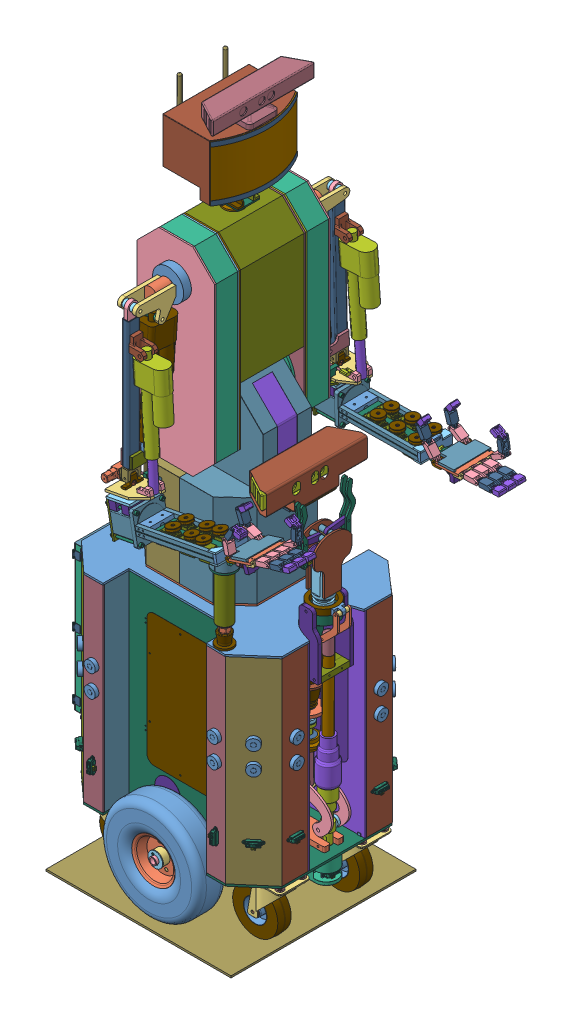
SolidWorks assembly sorbot, configuration По умолчанию. Lengths in mm.
Overall size (793.33 1880.98 665.85).
1182 component instances, 374 part files, 1522 mates.
Components (placement in the parent):
- wheel-1: wheel [По умолчанию] at (-13.022 1.4469 17.7637) size (270 270 80)
  - wheel.chamber-1: wheel.chamber [По умолчанию] at (6.3301 10.4899 0) size (270 270 80)
  - wheel.metal.front-1: wheel.metal.front [По умолчанию] at (6.3301 10.4899 42.7077) x (-0.311346 0.950297 0) z (0.950297 0.311346 0) size (117.48 26.95 117.48)
  - wheel.metal.internal-1: wheel.metal.internal [По умолчанию] at (6.3301 10.4899 36.3681) x (0.950297 0.311346 0) z (-0.311346 0.950297 0) size (117.48 60 117.48)
- wheel-2: wheel [По умолчанию] at (1.0599 2.4489 -290) x (-0.989924 -0.141601 0) z (0 0 -1) size (270 270 80)
  - wheel.chamber-1: wheel.chamber [По умолчанию] at (6.3301 10.4899 0) size (270 270 80)
  - wheel.metal.front-1: wheel.metal.front [По умолчанию] at (6.3301 10.4899 42.7077) x (-0.311346 0.950297 0) z (0.950297 0.311346 0) size (117.48 26.95 117.48)
  - wheel.metal.internal-1: wheel.metal.internal [По умолчанию] at (6.3301 10.4899 36.3681) x (0.950297 0.311346 0) z (-0.311346 0.950297 0) size (117.48 60 117.48)
- wheel.axis-1: wheel.axis [По умолчанию] at (-6.6918 11.9368 88.1319) x (-0.923728 -0.383049 0) z (0 0 -1) size (20 20 450)
- wheel.washer-1: wheel.washer [По умолчанию] at (-6.6918 11.9368 79.1319) size (40 40 2)
- wheel.washer-2: wheel.washer [По умолчанию] at (-6.6918 11.9368 -353.3681) size (40 40 2)
- wheel.axis.splint-1: wheel.axis.splint [По умолчанию] at (-51.8409 -4.2239 -121.73) x (0.909121 0.380793 -0.168805) z (0.181229 0.003281 0.983435) size (4.99 27.52 1.94)
- wheel.axis.splint-2: wheel.axis.splint [По умолчанию] at (-119.6931 -47.4576 -189.7376) x (-0.699932 -0.282835 -0.65582) z (0.605814 0.251217 -0.754904) size (4.99 27.52 1.94)
- wheel.disk-1: wheel.disk [По умолчанию] at (-6.6918 11.9368 -326.3681) size (86 86 70)
- gearmotor-1: gearmotor [По умолчанию] at (53.2168 119.2767 -131.0001) x (0.993251 -0.115983 0) z (0 0 1) size (79 79 282)
- wheel.bearing-1: wheel.bearing [По умолчанию] at (-6.6918 11.9368 -263.3681) x (0.993854 -0.110698 0) z (0 0 1) size (32 32 7)
- wheel.stop.bearing-2: wheel.stop.bearing [По умолчанию] at (-3.289 9.2452 -250.3457) size (52.27 52.27 14.02)
  - wheel.stop.bearing.p1-1: wheel.stop.bearing.p1 [По умолчанию] at (-3.4029 2.6916 -6.0224) size (40 40 4)
  - wheel.stop.bearing.p2-1: wheel.stop.bearing.p2 [По умолчанию] at (-3.421 17.5634 1.5621) size (7 7 7)
  - wheel.stop.bearing.p1-2: wheel.stop.bearing.p1 [По умолчанию] at (-3.4029 2.6916 8) x (-0.923728 -0.383049 0) z (0 0 -1) size (40 40 4)
  - wheel.stop.bearing.p2-3: wheel.stop.bearing.p2 [По умолчанию] at (4.0173 15.58 1.5621) x (0.866025 -0.5 0) z (0 0 1) size (7 7 7)
  - wheel.stop.bearing.p2-4: wheel.stop.bearing.p2 [По умолчанию] at (9.4674 10.1432 1.5621) x (0.5 -0.866025 0) z (0 0 1) size (7 7 7)
  - wheel.stop.bearing.p2-5: wheel.stop.bearing.p2 [По умолчанию] at (11.469 2.7097 1.5621) x (0 -1 0) z (0 0 1) size (7 7 7)
  - wheel.stop.bearing.p2-6: wheel.stop.bearing.p2 [По умолчанию] at (9.4856 -4.7286 1.5621) x (-0.5 -0.866025 0) z (0 0 1) size (7 7 7)
  - wheel.stop.bearing.p2-7: wheel.stop.bearing.p2 [По умолчанию] at (4.0488 -10.1787 1.5621) x (-0.866025 -0.5 0) z (0 0 1) size (7 7 7)
  - wheel.stop.bearing.p2-8: wheel.stop.bearing.p2 [По умолчанию] at (-3.3847 -12.1802 1.5621) x (-1 0 0) z (0 0 1) size (7 7 7)
  - wheel.stop.bearing.p2-9: wheel.stop.bearing.p2 [По умолчанию] at (-10.8231 -10.1969 1.5621) x (-0.866025 0.5 0) z (0 0 1) size (7 7 7)
  - wheel.stop.bearing.p2-10: wheel.stop.bearing.p2 [По умолчанию] at (-16.2732 -4.76 1.5621) x (-0.5 0.866025 0) z (0 0 1) size (7 7 7)
  - wheel.stop.bearing.p2-11: wheel.stop.bearing.p2 [По умолчанию] at (-18.2747 2.6734 1.5621) x (0 1 0) z (0 0 1) size (7 7 7)
  - wheel.stop.bearing.p2-12: wheel.stop.bearing.p2 [По умолчанию] at (-16.2913 10.1118 1.5621) x (0.5 0.866025 0) z (0 0 1) size (7 7 7)
  - wheel.stop.bearing.p2-13: wheel.stop.bearing.p2 [По умолчанию] at (-10.8545 15.5619 1.5621) x (0.866025 0.5 0) z (0 0 1) size (7 7 7)
- sproket.initial-1: sproket.initial [По умолчанию] at (53.2168 119.2767 -271.5001) x (0.999977 0.00678 0) z (0 0 1) size (82.09 81.83 4.4)
- gearmotor.sprocket.wheel.disk-1: gearmotor.sprocket.wheel.disk [По умолчанию] at (53.2168 119.2767 -276.8747) x (0.999997 -0.002459 0) z (0 0 1) size (68 68 28.87)
- sprocket-1: sprocket [По умолчанию] at (-6.6918 11.9368 -271.3681) size (82.09 81.83 3)
- bottom-2: bottom [По умолчанию] at (-6.1674 46.4368 -211.0406) size (543.13 5.5 438.63)
- wheel.axis.frame-3: wheel.axis.frame [По умолчанию] at (43.3082 10.4368 -242.3457) x (-1 0 0) z (0 0 1) size (126 65.5 38)
- accumulator1-1: accumulator1 [По умолчанию] at (-188.4596 154.9368 -137.8821) x (0 0 1) z (-1 0 0) size (232 218.1 175)
- wheel.disk-2: wheel.disk [По умолчанию] at (-6.6918 11.9368 54.1319) x (-0.923728 -0.383049 0) z (0 0 -1) size (86 86 70)
- wheel.bearing-2: wheel.bearing [По умолчанию] at (-6.6918 11.9368 -15.8681) size (32 32 7)
- wheel.stop.bearing-3: wheel.stop.bearing [По умолчанию] at (-3.289 9.2452 -23.8681) size (52.27 52.27 14.02)
  - wheel.stop.bearing.p1-1: wheel.stop.bearing.p1 [По умолчанию] at (-3.4029 2.6916 -6.0224) size (40 40 4)
  - wheel.stop.bearing.p2-1: wheel.stop.bearing.p2 [По умолчанию] at (-3.421 17.5634 1.5621) size (7 7 7)
  - wheel.stop.bearing.p1-2: wheel.stop.bearing.p1 [По умолчанию] at (-3.4029 2.6916 8) x (-0.923728 -0.383049 0) z (0 0 -1) size (40 40 4)
  - wheel.stop.bearing.p2-3: wheel.stop.bearing.p2 [По умолчанию] at (4.0173 15.58 1.5621) x (0.866025 -0.5 0) z (0 0 1) size (7 7 7)
  - wheel.stop.bearing.p2-4: wheel.stop.bearing.p2 [По умолчанию] at (9.4674 10.1432 1.5621) x (0.5 -0.866025 0) z (0 0 1) size (7 7 7)
  - wheel.stop.bearing.p2-5: wheel.stop.bearing.p2 [По умолчанию] at (11.469 2.7097 1.5621) x (0 -1 0) z (0 0 1) size (7 7 7)
  - wheel.stop.bearing.p2-6: wheel.stop.bearing.p2 [По умолчанию] at (9.4856 -4.7286 1.5621) x (-0.5 -0.866025 0) z (0 0 1) size (7 7 7)
  - wheel.stop.bearing.p2-7: wheel.stop.bearing.p2 [По умолчанию] at (4.0488 -10.1787 1.5621) x (-0.866025 -0.5 0) z (0 0 1) size (7 7 7)
  - wheel.stop.bearing.p2-8: wheel.stop.bearing.p2 [По умолчанию] at (-3.3847 -12.1802 1.5621) x (-1 0 0) z (0 0 1) size (7 7 7)
  - wheel.stop.bearing.p2-9: wheel.stop.bearing.p2 [По умолчанию] at (-10.8231 -10.1969 1.5621) x (-0.866025 0.5 0) z (0 0 1) size (7 7 7)
  - wheel.stop.bearing.p2-10: wheel.stop.bearing.p2 [По умолчанию] at (-16.2732 -4.76 1.5621) x (-0.5 0.866025 0) z (0 0 1) size (7 7 7)
  - wheel.stop.bearing.p2-11: wheel.stop.bearing.p2 [По умолчанию] at (-18.2747 2.6734 1.5621) x (0 1 0) z (0 0 1) size (7 7 7)
  - wheel.stop.bearing.p2-12: wheel.stop.bearing.p2 [По умолчанию] at (-16.2913 10.1118 1.5621) x (0.5 0.866025 0) z (0 0 1) size (7 7 7)
  - wheel.stop.bearing.p2-13: wheel.stop.bearing.p2 [По умолчанию] at (-10.8545 15.5619 1.5621) x (0.866025 0.5 0) z (0 0 1) size (7 7 7)
- wheel.axis.frame-4: wheel.axis.frame [По умолчанию] at (-56.6918 10.4368 -29.8906) x (1 0 0) z (0 0 -1) size (126 65.5 38)
- sprocket-2: sprocket [По умолчанию] at (-6.6918 11.9368 -3.8681) x (0.99994 0.010997 0) z (0 0 1) size (82.09 81.83 3)
- gearmotor-2: gearmotor [По умолчанию] at (-40.8776 119.0545 -142.1692) x (-0.999846 -0.017524 0) z (0 0 -1) size (79 79 282)
- gearmotor.sprocket.wheel.disk-2: gearmotor.sprocket.wheel.disk [По умолчанию] at (-40.8776 119.0545 3.7054) x (-0.999846 -0.017524 0) z (0 0 -1) size (68 68 28.87)
- sproket.initial-2: sproket.initial [По умолчанию] at (-40.8776 119.0545 -1.6692) x (-0.999994 -0.003421 0) z (0 0 -1) size (82.09 81.83 4.4)
- man1-2: man1 [По умолчанию] at (221.423 424.2117 -133.5351) x (0 0 -1) z (1 0 0) size (154.52 823.81 284.97)
  - man1.actuator-1: man1.actuator [По умолчанию] at (-0.3986 -205.8789 -139.5078) x (-1 0 0) z (0 1 0.000021) size (65 65 317.39)
    - man1.drive1-1: man1.drive1 [По умолчанию] at (-4.1866 0.6029 0) size (50 50 148.25)
    - man1.drive1.frame.p1-1: man1.drive1.frame.p1 [По умолчанию] at (-4.1866 0.6029 121) size (28 28 8)
    - man1.drive1.frame.p2-1: man1.drive1.frame.p2 [По умолчанию] at (-4.1866 0.6029 121) size (65 65 8)
    - man1.drive1.frame.p4-1: man1.drive1.frame.p4 [По умолчанию] at (-4.1866 0.6029 -33) size (54 65 20)
    - man1.drive1.frame.p5-1: man1.drive1.frame.p5 [По умолчанию] at (-4.1866 0.6029 -37.3912) x (0.999995 0.003021 0) z (0 0 1) size (41.77 41.77 245)
    - man1.drive1.frame.p6-1: man1.drive1.frame.p6 [По умолчанию] at (-4.1866 0.6029 129) size (30 30 25)
    - man1.drive1.frame.p7-1: man1.drive1.frame.p7 [По умолчанию] at (-4.1866 0.6029 154) size (30 30 2)
    - man1.drive1.frame.p8-1: man1.drive1.frame.p8 [По умолчанию] at (-4.1866 0.6029 156) size (30 30 28)
    - man1.drive1.frame.p10-1: man1.drive1.frame.p10 [По умолчанию] at (-4.1866 0.6029 164) size (10.5 10.5 116)
    - man1.drive1.frame.p9-1: man1.drive1.frame.p9 [По умолчанию] at (-4.1866 0.6029 187) size (65 65 28)
    - man1.drive1.frame.p11-1: man1.drive1.frame.p11 [По умолчанию] at (-4.1866 0.6029 187) size (35 35 24)
    - man1.drive1.frame.p3-7: man1.drive1.frame.p3 [По умолчанию] at (-4.1866 0.6029 58) size (65 65 5)
  - man1.p1-1: man1.p1 [По умолчанию] at (52.788 -228.8789 -138.9054) x (-1 0 0) z (0 0 1) size (100 8 8)
  - man1.drive1.frame.p12-1: man1.drive1.frame.p12 [По умолчанию] at (3.788 68.5641 -138.8992) x (-1 0 0) z (0 1 0.000021) size (21 21 93.41)
  - man1.p2-1: man1.p2 [По умолчанию] at (-22.212 -237.9208 -123.0814) x (0 0 -1) z (-1 0 0) size (72.27 30 90)
  - man1.p5-1: man1.p5 [По умолчанию] at (4.7507 160.9388 -85.9149) x (-1 0 0) z (0 -0.002225 0.999998) size (26 90 26)
  - man1.p4-1: man1.p4 [По умолчанию] at (3.7914 125.9389 -85.9928) x (0.93549 0.000786 -0.353351) z (-0.353352 0.002082 -0.935488) size (30 487 30)
  - man1.p3-2: man1.p3 [По умолчанию] at (38.7914 154.9807 -70.1243) x (0 0 -1) z (1 0 0) size (125.25 30 85)
  - man1.p6-1: man1.p6 [По умолчанию] at (42.008 145.9388 -85.9483) x (-1 0 0) z (0 0.364371 -0.931254) size (75 8 8)
  - man1.p7-2: man1.p7 [По умолчанию] at (23.8722 69.7096 -67.4428) x (-1 0 0) z (0 -0.002225 0.999998) size (74 91.83 135.45)
  - man1.actuator-2: man1.actuator [По умолчанию] at (8.0554 58.0922 -32.4461) x (1 0 0) z (0 -0.999998 -0.002148) size (65 65 317.39)
    - man1.drive1-1: man1.drive1 [По умолчанию] at (-4.1866 0.6029 0) size (50 50 148.25)
    - man1.drive1.frame.p1-1: man1.drive1.frame.p1 [По умолчанию] at (-4.1866 0.6029 121) size (28 28 8)
    - man1.drive1.frame.p2-1: man1.drive1.frame.p2 [По умолчанию] at (-4.1866 0.6029 121) size (65 65 8)
    - man1.drive1.frame.p4-1: man1.drive1.frame.p4 [По умолчанию] at (-4.1866 0.6029 -33) size (54 65 20)
    - man1.drive1.frame.p5-1: man1.drive1.frame.p5 [По умолчанию] at (-4.1866 0.6029 -37.3912) x (0.999995 0.003021 0) z (0 0 1) size (41.77 41.77 245)
    - man1.drive1.frame.p6-1: man1.drive1.frame.p6 [По умолчанию] at (-4.1866 0.6029 129) size (30 30 25)
    - man1.drive1.frame.p7-1: man1.drive1.frame.p7 [По умолчанию] at (-4.1866 0.6029 154) size (30 30 2)
    - man1.drive1.frame.p8-1: man1.drive1.frame.p8 [По умолчанию] at (-4.1866 0.6029 156) size (30 30 28)
    - man1.drive1.frame.p10-1: man1.drive1.frame.p10 [По умолчанию] at (-4.1866 0.6029 164) size (10.5 10.5 116)
    - man1.drive1.frame.p9-1: man1.drive1.frame.p9 [По умолчанию] at (-4.1866 0.6029 187) size (65 65 28)
    - man1.drive1.frame.p11-1: man1.drive1.frame.p11 [По умолчанию] at (-4.1866 0.6029 187) size (35 35 24)
    - man1.drive1.frame.p3-7: man1.drive1.frame.p3 [По умолчанию] at (-4.1866 0.6029 58) size (65 65 5)
  - man1.drive1.frame.p12-2: man1.drive1.frame.p12 [По умолчанию] at (3.8689 -153.2296 -32.2971) x (1 0 0) z (0 -0.999998 -0.002148) size (21 21 93.41)
  - man1.p8-1: man1.p8 [По умолчанию] at (3.7914 -359.7465 -87.0735) x (0 -0.002225 0.999998) z (-1 0 0) size (145 30 54.24)
  - man1.p11-2: man1.p11 [По умолчанию] at (-11.2086 -199.8321 18.3244) x (-1 0 0) z (0 0.071625 0.997432) size (5.5 105.72 90.08)
  - man1.p12-2: man1.p12 [По умолчанию] at (-22.7871 -224.5214 -51.2659) x (1 0 0) z (0 0.19273 0.981252) size (5.5 118.7 99.86)
  - man1.p13-1: man1.p13 [По умолчанию] at (-4.1311 -234.2294 -32.471) x (1 0 0) z (0 -0.069887 -0.997555) size (7 26 26)
  - man1.p13-2: man1.p13 [По умолчанию] at (-10.2871 -314.4644 20.4089) x (1 0 0) z (0 0 1) size (7 26 26)
  - man1.p13-3: man1.p13 [По умолчанию] at (18.8689 -234.2294 -32.471) size (7 26 26)
  - man1.p12-3: man1.p12 [По умолчанию] at (24.7129 -224.5214 -51.2659) x (1 0 0) z (0 0.19273 0.981252) size (5.5 118.7 99.86)
  - man1.p13-4: man1.p13 [По умолчанию] at (24.7129 -314.4644 20.4089) x (1 0 0) z (0 -0.270753 0.962649) size (7 26 26)
  - man1.drive2-1: man1.drive2 [По умолчанию] at (3.7079 -240.2809 21.0583) x (0.972815 -0.000504 0.231584) z (0 0.999998 0.002174) size (32 32 80.98)
  - man1.p14-1: man1.p14 [По умолчанию] at (3.7079 -243.1669 21.052) x (0.999283 0.000082 -0.03786) z (0.03786 -0.002173 0.999281) size (50 191 50)
  - man1.p15-1: man1.p15 [По умолчанию] at (3.7079 -218.9022 21.1047) x (0.998805 0.000106 -0.048869) z (0.048869 -0.002172 0.998803) size (52 118 52)
  - man1.p16-1: man1.p16 [По умолчанию] at (3.7079 -152.1041 21.25) x (0.992237 0.00027 -0.124359) z (0.12436 -0.002157 0.992235) size (24.7 240 24.7)
  - man1.p17-1: man1.p17 [По умолчанию] at (3.7079 -169.2808 21.2126) x (0.999945 0.000023 -0.010535) z (0.010535 -0.002174 0.999942) size (23 37 23)
  - man1.p18-1: man1.p18 [По умолчанию] at (3.7079 -154.5438 21.2447) x (0.916473 0.00087 -0.400097) z (0.400098 -0.001993 0.91647) size (10 240 10)
  - man1.stok.2-1: man1.stok.2 [По умолчанию] at (4.7586 51.1132 21.6972) x (0.999987 -0.000011 0.005102) z (-0.005102 -0.002174 0.999985) size (31.92 103 31.92)
    - man1.p19-1: man1.p19 [По умолчанию] at (-1.0508 -2.675 0) x (1 0 -0.000645) z (0.000645 0 1) size (14 6 15.86)
    - man1.p20-1: man1.p20 [По умолчанию] at (-1.0508 -12.2265 0) x (0.999987 0 -0.005102) z (0.005102 0 0.999987) size (24 100 24)
    - man1.p19-2: man1.p19 [По умолчанию] at (-1.0508 -9.0548 0) x (1 0 -0.000645) z (0.000645 0 1) size (14 6 15.86)
    - man1.p21-1: man1.p21 [По умолчанию] at (-1.0508 -8.2265 0) x (-0.905374 0 -0.424616) z (-0.424616 0 0.905374) size (24 7 24)
  - man1.drive3-1: man1.drive3 [По умолчанию] at (3.7079 171.7029 8.9923) x (-0.018472 -0.002174 0.999827) z (-0.999829 0.00004 -0.018472) size (76 103.5 76)
  - man1.p22-1: man1.p22 [По умолчанию] at (3.7079 46.078 21.6809) x (0 -0.002174 0.999998) z (-1 0 0) size (20 15 76)
  - man1.p22-2: man1.p22 [По умолчанию] at (3.7079 46.078 21.6809) x (0 0.002174 -0.999998) z (1 0 0) size (20 15 76)
  - man1.p23-1: man1.p23 [По умолчанию] at (-44.2921 76.2218 21.7464) x (1 0 0) z (0 -0.002174 0.999998) size (10 166.6 51.35)
  - man1.p24-1: man1.p24 [По умолчанию] at (3.7079 194.7029 9.0423) x (1 0 0) z (0 -0.002174 0.999998) size (76 16 76)
  - man1.p25-1: man1.p25 [По умолчанию] at (3.7079 188.7029 9.0293) x (1 0 0) z (0 -0.002174 0.999998) size (30 16 20.8)
  - man1.p26-2: man1.p26 [По умолчанию] at (-14.0001 197.4558 58.3526) x (1 0 0) z (0 -0.797207 0.603707) size (5 86.81 49.56)
  - man1.p27-1: man1.p27 [По умолчанию] at (-11.2921 202.5951 58.6309) x (1 0 0) z (0 0 1) size (10 12 12)
  - man1.p23-2: man1.p23 [По умолчанию] at (41.7079 76.2218 21.7464) x (1 0 0) z (0 -0.002174 0.999998) size (10 166.6 51.35)
  - man1.p26-3: man1.p26 [По умолчанию] at (18.7079 197.4558 58.3526) x (1 0 0) z (0 -0.797207 0.603707) size (5 86.81 49.56)
  - man1.p27-2: man1.p27 [По умолчанию] at (8.7079 202.5951 58.6309) x (1 0 0) z (0 0 1) size (10 12 12)
  - man1.p28-1: man1.p28 [По умолчанию] at (3.7079 199.7029 9.0532) x (1 0 0) z (0 -0.002174 0.999998) size (44 5 44)
  - man1.p29-1: man1.p29 [По умолчанию] at (3.7079 204.7029 9.0641) x (1 0 0) z (0 -0.002174 0.999998) size (48 87 48)
  - man1.drive4-2: man1.drive4 [По умолчанию] at (3.7079 223.5144 9.105) x (1 0 0) z (0 0.999998 0.002174) size (32 32 76.8)
  - man1.p30-1: man1.p30 [По умолчанию] at (3.7079 306.0105 9.2843) x (1 0 0) z (0 -0.002174 0.999998) size (9 22 9.04)
  - man1.p31-1: man1.p31 [По умолчанию] at (29.5403 324.041 7.7213) x (-0.983063 0.183268 0.000398) z (0 -0.002174 0.999998) size (45 45 3.2)
  - man1.p32-1: man1.p32 [По умолчанию] at (3.7079 291.7765 9.2534) x (0.999646 0.000058 -0.02662) z (0.02662 -0.002173 0.999643) size (7 52 7)
  - man1.p31-2: man1.p31 [По умолчанию] at (-22.1256 324.041 7.7213) x (0.982203 0.187824 0.000408) z (0 -0.002174 0.999998) size (45 45 3.2)
  - man1.p33-1: man1.p33 [По умолчанию] at (3.7079 339.6174 9.3574) x (1 0 -0.000001) z (0.000001 -0.002174 0.999998) size (11 4 11)
  - man1.p34-1: man1.p34 [По умолчанию] at (3.917 260.5145 29.2177) x (1 0 0) z (0 -0.002174 0.999998) size (102 143.82 5)
  - man1.p35-1: man1.p35 [По умолчанию] at (3.5428 345.6669 -0.5972) x (1 0 0) z (0 -0.002174 0.999998) size (21.92 13.34 40.06)
  - man1.p34-2: man1.p34 [По умолчанию] at (3.9108 260.6834 -15.8465) x (1 0 0) z (0 -0.002174 0.999998) size (102 143.82 5)
  - man1.p36-1: man1.p36 [По умолчанию] at (-22.1256 324.3066 -114.43) x (-0.911615 -0.411045 -0.000894) z (-0.411046 0.911612 0.001982) size (14 12.53 14)
  - man1.p36-4: man1.p36 [По умолчанию] at (29.5403 323.8283 105.543) x (1 0 0) z (0 0.999998 0.002174) size (14 12.53 14)
  - man1.p36-5: man1.p36 [По умолчанию] at (-22.1256 324.2467 -86.8959) x (0.923728 0.383048 0.000833) z (0.383049 -0.923726 -0.002008) size (14 12.53 14)
  - man1.p36-6: man1.p36 [По умолчанию] at (29.5403 324.2467 -86.8955) x (0.923728 0.383048 0.000833) z (0.383049 -0.923726 -0.002008) size (14 12.53 14)
  - man1.p39-1: man1.p39 [По умолчанию] at (-8.83 360.2475 -10.63) x (1 0 0) z (0 -0.002174 0.999998) size (14 14 15)
  - man1.p39-2: man1.p39 [По умолчанию] at (-8.83 360.193 14.4344) x (-0.43245 -0.901656 -0.00196) z (0 -0.002174 0.999998) size (14 14 15)
  - man1.p40-1: man1.p40 [По умолчанию] at (-55.263 317.6909 13.8075) x (0.999938 0.011102 0.000024) z (0 -0.002174 0.999998) size (24.21 150.81 5)
  - man1.p37-2: man1.p37 [По умолчанию] at (29.5403 324.0538 1.8213) x (-0.983063 0.183268 0.000398) z (0 -0.002174 0.999998) size (47.74 16 15)
  - man1.p37-3: man1.p37 [По умолчанию] at (-22.1256 324.0538 1.8213) x (0.982203 0.187824 0.000408) z (0 -0.002174 0.999998) size (47.74 16 15)
  - man1.p38-3: man1.p38 [По умолчанию] at (-20.7361 362.973 4.9059) x (0.932121 -0.362146 -0.000787) z (0 -0.002174 0.999998) size (59.39 24.42 8)
  - man1.p40-5: man1.p40 [По умолчанию] at (-55.263 317.7214 -0.1925) x (0.999938 0.011102 0.000024) z (0 -0.002174 0.999998) size (24.21 150.81 5)
  - man1.p39-5: man1.p39 [По умолчанию] at (15.9138 360.2483 -10.63) x (1 0 0) z (0 -0.002174 0.999998) size (14 14 15)
  - man1.p40-6: man1.p40 [По умолчанию] at (62.7068 317.8338 18.8078) x (-0.999994 0.003344 0.000007) z (0 0.002174 -0.999998) size (24.21 150.81 5)
  - man1.p40-7: man1.p40 [По умолчанию] at (62.7068 317.8642 4.8078) x (-0.999994 0.003344 0.000007) z (0 0.002174 -0.999998) size (24.21 150.81 5)
  - man1.p38-4: man1.p38 [По умолчанию] at (28.1093 361.0126 4.9017) x (-0.996999 0.077416 0.000168) z (0 -0.002174 0.999998) size (59.39 24.42 8)
  - man1.p39-6: man1.p39 [По умолчанию] at (15.9138 360.1938 14.4344) x (1 0 0) z (0 -0.002174 0.999998) size (14 14 15)
  - man1.p11-4: man1.p11 [По умолчанию] at (18.7914 -373.8941 -100.5086) x (1 0 0) z (0 -0.955022 0.296534) size (5.5 105.72 90.08)
- gearmotor-3: gearmotor [По умолчанию] at (-20.0648 476.1505 -136.9555) x (1 0 0) z (0 -1 0) size (79 79 282)
- wheel1-1: wheel1 [По умолчанию] at (-196.5272 -62.2972 -25.6616) x (-1 0 0) z (0 0 -1) size (200.34 170.67 200.34)
  - wheel1.p1-1: wheel1.p1 [По умолчанию] at (-12.811 1.8421 0) size (125 125 36)
  - wheel1.p2-1: wheel1.p2 [По умолчанию] at (-12.811 1.8421 0.314) size (63.07 63.07 18)
  - wheel1.p2-2: wheel1.p2 [По умолчанию] at (-12.811 1.8421 -1.8658) x (-0.923728 -0.383049 0) z (0 0 -1) size (63.07 63.07 18)
  - wheel1.p3-1: wheel1.p3 [По умолчанию] at (-12.811 1.8421 -23.186) size (26 26 45)
  - wheel1.p4-1: wheel1.p4 [По умолчанию] at (24.859 90.4164 -1.436) size (105.01 101.57 85.69)
  - wheel1.p5-1: wheel1.p5 [По умолчанию] at (-14.7105 107.5716 -31.4713) x (-0.835986 -0.053146 -0.546171) z (-0.546944 0 0.837169) size (19.35 16 19.35)
  - wheel1.p5-2: wheel1.p5 [По умолчанию] at (64.4343 107.3349 28.3568) x (-0.998587 -0.053146 0) z (0 0 1) size (19.35 16 19.35)
  - wheel1.p5-3: wheel1.p5 [По умолчанию] at (64.0198 107.4544 -30.9637) x (-0.998587 -0.053146 0) z (0 0 1) size (19.35 16 19.35)
  - wheel1.p5-4: wheel1.p5 [По умолчанию] at (-14.3812 94.4397 28.6561) x (0.835986 0.053146 0.546171) z (-0.546944 0 0.837169) size (19.35 16 19.35)
- gearmotor.fixture.p3-1: gearmotor.fixture.p3 [По умолчанию] at (-40.8776 119.0545 -206.1702) x (0.994905 -0.100817 0) z (0 0 1) size (85.63 69.7 25)
- gearmotor.fixture.p2-3: gearmotor.fixture.p2 [По умолчанию] at (10.2084 53.4933 -65.0001) size (86 101.43 182)
- gearmotor.fixture.p3-2: gearmotor.fixture.p3 [По умолчанию] at (53.2274 119.174 -90.4218) x (0.994792 -0.101924 0) z (0 0 1) size (85.63 69.7 25)
- wheel1-5: wheel1 [По умолчанию] at (187.6309 -62.2985 -24.8952) size (200.34 170.67 200.34)
  - wheel1.p1-1: wheel1.p1 [По умолчанию] at (-12.811 1.8421 0) size (125 125 36)
  - wheel1.p2-1: wheel1.p2 [По умолчанию] at (-12.811 1.8421 0.314) size (63.07 63.07 18)
  - wheel1.p2-2: wheel1.p2 [По умолчанию] at (-12.811 1.8421 -1.8658) x (-0.923728 -0.383049 0) z (0 0 -1) size (63.07 63.07 18)
  - wheel1.p3-1: wheel1.p3 [По умолчанию] at (-12.811 1.8421 -23.186) size (26 26 45)
  - wheel1.p4-1: wheel1.p4 [По умолчанию] at (24.859 90.4164 -1.436) size (105.01 101.57 85.69)
  - wheel1.p5-1: wheel1.p5 [По умолчанию] at (-14.7105 107.5716 -31.4713) x (-0.835986 -0.053146 -0.546171) z (-0.546944 0 0.837169) size (19.35 16 19.35)
  - wheel1.p5-2: wheel1.p5 [По умолчанию] at (64.4343 107.3349 28.3568) x (-0.998587 -0.053146 0) z (0 0 1) size (19.35 16 19.35)
  - wheel1.p5-3: wheel1.p5 [По умолчанию] at (64.0198 107.4544 -30.9637) x (-0.998587 -0.053146 0) z (0 0 1) size (19.35 16 19.35)
  - wheel1.p5-4: wheel1.p5 [По умолчанию] at (-14.3812 94.4397 28.6561) x (0.835986 0.053146 0.546171) z (-0.546944 0 0.837169) size (19.35 16 19.35)
- wheel1-7: wheel1 [По умолчанию] at (-196.1639 -62.2105 -250.4568) x (-1 0 0) z (0 0 -1) size (200.34 170.67 200.34)
  - wheel1.p1-1: wheel1.p1 [По умолчанию] at (-12.811 1.8421 0) size (125 125 36)
  - wheel1.p2-1: wheel1.p2 [По умолчанию] at (-12.811 1.8421 0.314) size (63.07 63.07 18)
  - wheel1.p2-2: wheel1.p2 [По умолчанию] at (-12.811 1.8421 -1.8658) x (-0.923728 -0.383049 0) z (0 0 -1) size (63.07 63.07 18)
  - wheel1.p3-1: wheel1.p3 [По умолчанию] at (-12.811 1.8421 -23.186) size (26 26 45)
  - wheel1.p4-1: wheel1.p4 [По умолчанию] at (24.859 90.4164 -1.436) size (105.01 101.57 85.69)
  - wheel1.p5-1: wheel1.p5 [По умолчанию] at (-14.7105 107.5716 -31.4713) x (-0.835986 -0.053146 -0.546171) z (-0.546944 0 0.837169) size (19.35 16 19.35)
  - wheel1.p5-2: wheel1.p5 [По умолчанию] at (64.4343 107.3349 28.3568) x (-0.998587 -0.053146 0) z (0 0 1) size (19.35 16 19.35)
  - wheel1.p5-3: wheel1.p5 [По умолчанию] at (64.0198 107.4544 -30.9637) x (-0.998587 -0.053146 0) z (0 0 1) size (19.35 16 19.35)
  - wheel1.p5-4: wheel1.p5 [По умолчанию] at (-14.3812 94.4397 28.6561) x (0.835986 0.053146 0.546171) z (-0.546944 0 0.837169) size (19.35 16 19.35)
- wheel1-8: wheel1 [По умолчанию] at (187.4476 -61.9053 -246.5204) size (200.34 170.67 200.34)
  - wheel1.p1-1: wheel1.p1 [По умолчанию] at (-12.811 1.8421 0) size (125 125 36)
  - wheel1.p2-1: wheel1.p2 [По умолчанию] at (-12.811 1.8421 0.314) size (63.07 63.07 18)
  - wheel1.p2-2: wheel1.p2 [По умолчанию] at (-12.811 1.8421 -1.8658) x (-0.923728 -0.383049 0) z (0 0 -1) size (63.07 63.07 18)
  - wheel1.p3-1: wheel1.p3 [По умолчанию] at (-12.811 1.8421 -23.186) size (26 26 45)
  - wheel1.p4-1: wheel1.p4 [По умолчанию] at (24.859 90.4164 -1.436) size (105.01 101.57 85.69)
  - wheel1.p5-1: wheel1.p5 [По умолчанию] at (-14.7105 107.5716 -31.4713) x (-0.835986 -0.053146 -0.546171) z (-0.546944 0 0.837169) size (19.35 16 19.35)
  - wheel1.p5-2: wheel1.p5 [По умолчанию] at (64.4343 107.3349 28.3568) x (-0.998587 -0.053146 0) z (0 0 1) size (19.35 16 19.35)
  - wheel1.p5-3: wheel1.p5 [По умолчанию] at (64.0198 107.4544 -30.9637) x (-0.998587 -0.053146 0) z (0 0 1) size (19.35 16 19.35)
  - wheel1.p5-4: wheel1.p5 [По умолчанию] at (-14.3812 94.4397 28.6561) x (0.835986 0.053146 0.546171) z (-0.546944 0 0.837169) size (19.35 16 19.35)
- wall1-1: wall1 [По умолчанию] at (26.1889 166.4368 -212.2424) x (0 0 1) z (-1 0 0) size (150 418.71 5)
- wall2-1: wall2 [По умолчанию] at (21.1889 166.4368 -62.2424) size (245.99 533.21 4)
- wall2-2: wall2 [По умолчанию] at (21.1889 166.4368 -216.2424) size (245.99 533.21 4)
- wall3-1: wall3 [По умолчанию] at (57.626 166.4368 -212.2424) x (0 0 1) z (-1 0 0) size (150 5 80.99)
- wall4-1: wall4 [По умолчанию] at (102.1741 112.2872 -162.1841) size (5 115 160)
- wall6-1: wall6 [По умолчанию] at (262.1742 51.9368 -58.2424) size (4 533.21 70.07)
- wall7-1: wall7 [По умолчанию] at (263.5274 51.9368 8.4769) x (0.650583 0 0.759435) z (-0.759435 0 0.650583) size (4 533.21 108.33)
- wall6-3: wall6 [По умолчанию] at (262.1741 51.9368 -286.3112) size (4 533.21 70.07)
- wall7-3: wall7 [По умолчанию] at (182.0437 51.9368 -352.0328) x (0.650583 0 -0.759435) z (0.759435 0 0.650583) size (4 533.21 108.33)
- wall8-1: wall8 [По умолчанию] at (184.9222 585.1368 77.4378) x (-0.999982 0 -0.006017) z (-0.006017 0 0.999982) size (52.1 533.2 4)
- wall8-2: wall8 [По умолчанию] at (132.798 585.1368 -351.1821) x (1 0 0) z (0 0 -1) size (52.1 533.2 4)
- wall9-1: wall9 [По умолчанию] at (131.9009 51.9368 18.6982) size (4 533.21 69.9)
- wall10-1: wall10 [По умолчанию] at (-1.8874 51.9368 6.1109) size (279.58 533.21 4)
- wall9-2: wall9 [По умолчанию] at (-151.6756 51.9368 18.7781) size (4 533.21 69.9)
- wall8-4: wall8 [По умолчанию] at (-146.6756 585.1505 77.4522) x (-1 0 0) z (0 0 1) size (52.1 533.2 4)
- wall7-v1-1: wall7-v1 [По умолчанию] at (-275.291 585.1505 5.6816) x (-0.67421 0 0.73854) z (0.73854 0 0.67421) size (4 533.21 104.08)
- wall11-1: wall11 [По умолчанию] at (-275.9003 51.4368 11.9312) size (4 556.08 297.39)
- wall7-v1-2: wall7-v1 [По умолчанию] at (-192.6496 585.1505 -354.9488) x (-0.67421 0 -0.73854) z (-0.73854 0 0.67421) size (4 533.21 104.08)
- wall8-5: wall8 [По умолчанию] at (-199.1911 585.1368 -351.1821) x (1 0 0) z (0 0 -1) size (52.1 533.2 4)
- wall9-3: wall9 [По умолчанию] at (-151.7539 51.9368 -346.0339) size (4 533.21 69.9)
- wall10-v1-1: wall10-v1 [По умолчанию] at (-11.9655 51.9368 -280.8407) x (-1 0 0) z (0 0 -1) size (279.58 533.21 4)
- wall9-4: wall9 [По умолчанию] at (131.8227 51.9368 -346.0339) size (4 533.21 69.9)
- cap-1: cap [По умолчанию] at (-5.7427 585.1505 -210.9644) x (0.999999 0 0.001245) z (-0.001245 0 0.999999) size (543.13 5 440.03)
- wall-fixture-v1-1: wall-fixture-v1 [По умолчанию] at (-173.7475 76.9368 76.4353) x (0 0 -1) z (1 0 0) size (22 468 22)
- wall-fixture-v2-1: wall-fixture-v2 [По умолчанию] at (-193.2465 76.9434 77.0334) x (1 0.000217 -0.000757) z (0.000757 0.000198 1) size (36.03 468.21 15.37)
- wall-fixture-v2-1-1: wall-fixture-v2-1 [По умолчанию] at (-267.8848 76.9368 11.8294) x (0.742362 0 0.669999) z (-0.669999 0 0.742362) size (35.21 468.21 16.9)
- wall-fixture-v1-2: wall-fixture-v1 [По умолчанию] at (-129.6037 76.9368 8.4522) x (0 0 1) z (-1 0 0) size (22 468 22)
- wall-fixture-v2-1-2: wall-fixture-v2-1 [По умолчанию] at (-270.3872 76.8439 -279.8709) x (0 0 1) z (-1 0 0) size (35.21 468.21 16.9)
- wall-fixture-v2-2: wall-fixture-v2 [По умолчанию] at (-198.9245 51.4368 -348.5071) x (-0.738029 0 0.674769) z (-0.674769 0 -0.738029) size (36.03 468.21 15.37)
- wall-fixture-v1-3: wall-fixture-v1 [По умолчанию] at (-152.8245 51.4368 -329.0518) x (-1 0 0) z (0 0 -1) size (22 468 22)
- wall-fixture-v1-4: wall-fixture-v1 [По умолчанию] at (-150.8245 51.4368 -303.2005) size (22 468 22)
- wall-fixture-v1-5: wall-fixture-v1 [По умолчанию] at (115.6802 51.4368 -282.1286) x (0 0 -1) z (1 0 0) size (22 468 22)
- wall-fixture-v1-6: wall-fixture-v1 [По умолчанию] at (159.8239 51.4368 -350.1821) x (0 0 1) z (-1 0 0) size (22 468 22)
- wall-fixture-v2-2-1: wall-fixture-v2-2 [По умолчанию] at (179.7171 51.4368 -350.669) x (-1 0 0) z (0 0 -1) size (37.63 460 15.83)
- wall-fixture-v2-3-1: wall-fixture-v2-3 [По умолчанию] at (259.0363 51.4368 -285.4128) x (-0.759435 0 -0.650583) z (0.650583 0 -0.759435) size (34.89 460 17.21)
- wall-fixture-v1-7: wall-fixture-v1 [По умолчанию] at (240.1022 51.4368 -218.2424) x (0 0 -1) z (1 0 0) size (22 468 22)
- wall-fixture-v1-8: wall-fixture-v1 [По умолчанию] at (261.1742 51.4368 -35.1705) x (-1 0 0) z (0 0 -1) size (22 468 22)
- wall-fixture-v2-4-1: wall-fixture-v2-4 [По умолчанию] at (259.1218 591.4368 11.3719) x (-0.758224 0 0.651995) z (0.651995 0 0.758224) size (34.89 460 17.21)
- wall-fixture-v2-5-1: wall-fixture-v2-5 [По умолчанию] at (178.2705 591.4368 76.9391) x (-1 0 0) z (0 0 1) size (37.63 460 15.83)
- wall-fixture-v1-9: wall-fixture-v1 [По умолчанию] at (138.9009 51.4368 55.3804) size (22 468 22)
- wall-fixture-v1-10: wall-fixture-v1 [По умолчанию] at (136.9009 76.9368 29.5241) x (-1 0 0) z (0 0 -1) size (22 468 22)
- wall-fixture-6-1: wall-fixture-6 [По умолчанию] at (79.1022 164.4368 -79.0844) x (0 -1 0) z (1 0 0) size (22 116 22)
- wall-fixture-6-2: wall-fixture-6 [По умолчанию] at (21.1889 187.5087 -195.3202) x (1 0 0) z (0 -1 0) size (22 116 22)
- wall-fixture-7-1: wall-fixture-7 [По умолчанию] at (21.2432 187.5087 -58.2424) x (0 0 -1) z (0 -1 0) size (22 81 22)
- wall-fixture-7-2: wall-fixture-7 [По умолчанию] at (102.2155 187.5087 -216.2424) x (0 0 1) z (0 -1 0) size (22 81 22)
- wall-fixture-8-1: wall-fixture-8 [По умолчанию] at (123.2459 51.3998 -216.2424) x (0 0 1) z (-1 0 0) size (22 112 22)
- wall-fixture-8-2: wall-fixture-8 [По умолчанию] at (102.1741 51.9112 -79.3142) size (22 112 22)
- wall-fixture-9-1: wall-fixture-9 [По умолчанию] at (21.1889 187.3953 -79.3142) size (22 390 22)
- wall-fixture-9-2: wall-fixture-9 [По умолчанию] at (42.2608 187.5289 -216.2424) x (0 0 1) z (-1 0 0) size (22 390 22)
- turret-1: turret [По умолчанию] at (-28.0267 628.2367 -136.0551) x (0.993667 0 -0.112365) z (0.112365 0 0.993667) size (200 17.64 200)
  - turret-p1-1: turret-p1 [По умолчанию] at (8.0127 -33.0433 0) size (180 12.6 180)
  - turret-p2-1: turret-p2 [По умолчанию] at (70.5799 -32.9814 -33.6477) size (10 10 10)
  - turret-p2-2: turret-p2 [По умолчанию] at (54.1999 -32.9814 -53.9774) x (0.932472 0 -0.361242) z (0.361242 0 0.932472) size (10 10 10)
  - turret-p2-3: turret-p2 [По умолчанию] at (31.5821 -32.9814 -67.0172) x (0.739009 0 -0.673696) z (0.673696 0 0.739009) size (10 10 10)
  - turret-p2-4: turret-p2 [По умолчанию] at (5.7811 -32.9814 -71.0059) x (0.445738 0 -0.895163) z (0.895163 0 0.445738) size (10 10 10)
  - turret-p2-5: turret-p2 [По умолчанию] at (-19.7185 -32.9814 -65.4049) x (0.092268 0 -0.995734) z (0.995734 0 0.092268) size (10 10 10)
  - turret-p2-6: turret-p2 [По умолчанию] at (-41.4728 -32.9814 -50.9706) x (-0.273663 0 -0.961826) z (0.961826 0 -0.273663) size (10 10 10)
  - turret-p2-7: turret-p2 [По умолчанию] at (-56.5439 -32.9814 -29.6524) x (-0.602635 0 -0.798017) z (0.798017 0 -0.602635) size (10 10 10)
  - turret-p2-8: turret-p2 [По умолчанию] at (-62.8962 -32.9814 -4.3296) x (-0.850217 0 -0.526432) z (0.526432 0 -0.850217) size (10 10 10)
  - turret-p2-9: turret-p2 [По умолчанию] at (-59.6719 -32.9814 21.5781) x (-0.982973 0 -0.18375) z (0.18375 0 -0.982973) size (10 10 10)
  - turret-p2-10: turret-p2 [По умолчанию] at (-47.3064 -32.9814 44.5714) x (-0.982973 0 0.18375) z (-0.18375 0 -0.982973) size (10 10 10)
  - turret-p2-11: turret-p2 [По умолчанию] at (-27.4698 -32.9814 61.5452) x (-0.850217 0 0.526432) z (-0.526432 0 -0.850217) size (10 10 10)
  - turret-p2-12: turret-p2 [По умолчанию] at (-2.8411 -32.9814 70.2069) x (-0.602635 0 0.798017) z (-0.798017 0 -0.602635) size (10 10 10)
  - turret-p2-13: turret-p2 [По умолчанию] at (23.2535 -32.9814 69.3868) x (-0.273663 0 0.961826) z (-0.961826 0 -0.273663) size (10 10 10)
  - turret-p2-14: turret-p2 [По умолчанию] at (47.2898 -32.9814 59.1957) x (0.092268 0 0.995734) z (-0.995734 0 0.092268) size (10 10 10)
  - turret-p2-15: turret-p2 [По умолчанию] at (66.0214 -32.9814 41.0098) x (0.445738 0 0.895163) z (-0.895163 0 0.445738) size (10 10 10)
  - turret-p2-16: turret-p2 [По умолчанию] at (76.9187 -32.9814 17.2853) x (0.739009 0 0.673696) z (-0.673696 0 0.739009) size (10 10 10)
  - turret-p2-17: turret-p2 [По умолчанию] at (78.5098 -32.9814 -8.7736) x (0.932472 0 0.361242) z (-0.361242 0 0.932472) size (10 10 10)
  - turret-p3-1: turret-p3 [По умолчанию] at (8.0127 -35.0433 0) x (0.999999 0 0.001108) z (-0.001108 0 0.999999) size (180 2 180)
  - turret-p5-1: turret-p5 [По умолчанию] at (92.4476 -23.6726 -1.2982) size (3 3 3)
  - turret-p5-2: turret-p5 [По умолчанию] at (92.1994 -23.6726 -6.5974) x (0.998027 0 -0.062791) z (0.062791 0 0.998027) size (3 3 3)
  - turret-p5-3: turret-p5 [По умолчанию] at (91.6191 -23.6726 -11.8705) x (0.992115 0 -0.125333) z (0.125333 0 0.992115) size (3 3 3)
  - turret-p5-4: turret-p5 [По умолчанию] at (90.7087 -23.6726 -17.0968) x (0.982287 0 -0.187381) z (0.187381 0 0.982287) size (3 3 3)
  - turret-p5-5: turret-p5 [По умолчанию] at (89.472 -23.6726 -22.2556) x (0.968583 0 -0.24869) z (0.24869 0 0.968583) size (3 3 3)
  - turret-p5-6: turret-p5 [По умолчанию] at (87.9138 -23.6726 -27.3265) x (0.951057 0 -0.309017) z (0.309017 0 0.951057) size (3 3 3)
  - turret-p5-7: turret-p5 [По умолчанию] at (86.0403 -23.6726 -32.2896) x (0.929776 0 -0.368125) z (0.368125 0 0.929776) size (3 3 3)
  - turret-p5-8: turret-p5 [По умолчанию] at (83.8589 -23.6726 -37.1253) x (0.904827 0 -0.425779) z (0.425779 0 0.904827) size (3 3 3)
  - turret-p5-9: turret-p5 [По умолчанию] at (81.3781 -23.6726 -41.8145) x (0.876307 0 -0.481754) z (0.481754 0 0.876307) size (3 3 3)
  - turret-p5-10: turret-p5 [По умолчанию] at (78.6078 -23.6726 -46.3386) x (0.844328 0 -0.535827) z (0.535827 0 0.844328) size (3 3 3)
  - turret-p5-11: turret-p5 [По умолчанию] at (75.5589 -23.6726 -50.6799) x (0.809017 0 -0.587785) z (0.587785 0 0.809017) size (3 3 3)
  - turret-p5-12: turret-p5 [По умолчанию] at (72.2433 -23.6726 -54.8211) x (0.770513 0 -0.637424) z (0.637424 0 0.770513) size (3 3 3)
  - turret-p5-13: turret-p5 [По умолчанию] at (68.6744 -23.6726 -58.746) x (0.728969 0 -0.684547) z (0.684547 0 0.728969) size (3 3 3)
  - turret-p5-14: turret-p5 [По умолчанию] at (64.866 -23.6726 -62.4391) x (0.684547 0 -0.728969) z (0.728969 0 0.684547) size (3 3 3)
  - turret-p5-15: turret-p5 [По умолчанию] at (60.8332 -23.6726 -65.8857) x (0.637424 0 -0.770513) z (0.770513 0 0.637424) size (3 3 3)
  - turret-p5-16: turret-p5 [По умолчанию] at (56.592 -23.6726 -69.0723) x (0.587785 0 -0.809017) z (0.809017 0 0.587785) size (3 3 3)
  - turret-p5-17: turret-p5 [По умолчанию] at (52.159 -23.6726 -71.9864) x (0.535827 0 -0.844328) z (0.844328 0 0.535827) size (3 3 3)
  - turret-p5-18: turret-p5 [По умолчанию] at (47.5518 -23.6726 -74.6163) x (0.481754 0 -0.876307) z (0.876307 0 0.481754) size (3 3 3)
  - turret-p5-19: turret-p5 [По умолчанию] at (42.7886 -23.6726 -76.9517) x (0.425779 0 -0.904827) z (0.904827 0 0.425779) size (3 3 3)
  - turret-p5-20: turret-p5 [По умолчанию] at (37.8882 -23.6726 -78.9835) x (0.368125 0 -0.929776) z (0.929776 0 0.368125) size (3 3 3)
  - turret-p5-21: turret-p5 [По умолчанию] at (32.8698 -23.6726 -80.7035) x (0.309017 0 -0.951057) z (0.951057 0 0.309017) size (3 3 3)
  - turret-p5-22: turret-p5 [По умолчанию] at (27.7533 -23.6726 -82.1051) x (0.24869 0 -0.968583) z (0.968583 0 0.24869) size (3 3 3)
  - turret-p5-23: turret-p5 [По умолчанию] at (22.559 -23.6726 -83.1826) x (0.187381 0 -0.982287) z (0.982287 0 0.187381) size (3 3 3)
  - turret-p5-24: turret-p5 [По умолчанию] at (17.3072 -23.6726 -83.9318) x (0.125333 0 -0.992115) z (0.992115 0 0.125333) size (3 3 3)
  - turret-p5-25: turret-p5 [По умолчанию] at (12.0187 -23.6726 -84.3498) x (0.062791 0 -0.998027) z (0.998027 0 0.062791) size (3 3 3)
  - turret-p5-26: turret-p5 [По умолчанию] at (6.7144 -23.6726 -84.4349) x (0 0 -1) z (1 0 0) size (3 3 3)
  - turret-p5-27: turret-p5 [По умолчанию] at (1.4153 -23.6726 -84.1868) x (-0.062791 0 -0.998027) z (0.998027 0 -0.062791) size (3 3 3)
  - turret-p5-28: turret-p5 [По умолчанию] at (-3.8578 -23.6726 -83.6064) x (-0.125333 0 -0.992115) z (0.992115 0 -0.125333) size (3 3 3)
  - turret-p5-29: turret-p5 [По умолчанию] at (-9.0841 -23.6726 -82.696) x (-0.187381 0 -0.982287) z (0.982287 0 -0.187381) size (3 3 3)
  - turret-p5-30: turret-p5 [По умолчанию] at (-14.2429 -23.6726 -81.4594) x (-0.24869 0 -0.968583) z (0.968583 0 -0.24869) size (3 3 3)
  - turret-p5-31: turret-p5 [По умолчанию] at (-19.3138 -23.6726 -79.9012) x (-0.309017 0 -0.951057) z (0.951057 0 -0.309017) size (3 3 3)
  - turret-p5-32: turret-p5 [По умолчанию] at (-24.2769 -23.6726 -78.0277) x (-0.368125 0 -0.929776) z (0.929776 0 -0.368125) size (3 3 3)
  - turret-p5-33: turret-p5 [По умолчанию] at (-29.1126 -23.6726 -75.8462) x (-0.425779 0 -0.904827) z (0.904827 0 -0.425779) size (3 3 3)
  - turret-p5-34: turret-p5 [По умолчанию] at (-33.8018 -23.6726 -73.3654) x (-0.481754 0 -0.876307) z (0.876307 0 -0.481754) size (3 3 3)
  - turret-p5-35: turret-p5 [По умолчанию] at (-38.3259 -23.6726 -70.5951) x (-0.535827 0 -0.844328) z (0.844328 0 -0.535827) size (3 3 3)
  - turret-p5-36: turret-p5 [По умолчанию] at (-42.6672 -23.6726 -67.5462) x (-0.587785 0 -0.809017) z (0.809017 0 -0.587785) size (3 3 3)
  - turret-p5-37: turret-p5 [По умолчанию] at (-46.8085 -23.6726 -64.2307) x (-0.637424 0 -0.770513) z (0.770513 0 -0.637424) size (3 3 3)
  - turret-p5-38: turret-p5 [По умолчанию] at (-50.7334 -23.6726 -60.6617) x (-0.684547 0 -0.728969) z (0.728969 0 -0.684547) size (3 3 3)
  - turret-p5-39: turret-p5 [По умолчанию] at (-54.4264 -23.6726 -56.8533) x (-0.728969 0 -0.684547) z (0.684547 0 -0.728969) size (3 3 3)
  - turret-p5-40: turret-p5 [По умолчанию] at (-57.873 -23.6726 -52.8205) x (-0.770513 0 -0.637424) z (0.637424 0 -0.770513) size (3 3 3)
  - turret-p5-41: turret-p5 [По умолчанию] at (-61.0597 -23.6726 -48.5793) x (-0.809017 0 -0.587785) z (0.587785 0 -0.809017) size (3 3 3)
  - turret-p5-42: turret-p5 [По умолчанию] at (-63.9737 -23.6726 -44.1463) x (-0.844328 0 -0.535827) z (0.535827 0 -0.844328) size (3 3 3)
  - turret-p5-43: turret-p5 [По умолчанию] at (-66.6036 -23.6726 -39.5392) x (-0.876307 0 -0.481754) z (0.481754 0 -0.876307) size (3 3 3)
  - turret-p5-44: turret-p5 [По умолчанию] at (-68.9391 -23.6726 -34.7759) x (-0.904827 0 -0.425779) z (0.425779 0 -0.904827) size (3 3 3)
  - turret-p5-45: turret-p5 [По умолчанию] at (-70.9708 -23.6726 -29.8755) x (-0.929776 0 -0.368125) z (0.368125 0 -0.929776) size (3 3 3)
  - turret-p5-46: turret-p5 [По умолчанию] at (-72.6908 -23.6726 -24.8571) x (-0.951057 0 -0.309017) z (0.309017 0 -0.951057) size (3 3 3)
  - turret-p5-47: turret-p5 [По умолчанию] at (-74.0924 -23.6726 -19.7407) x (-0.968583 0 -0.24869) z (0.24869 0 -0.968583) size (3 3 3)
  - turret-p5-48: turret-p5 [По умолчанию] at (-75.1699 -23.6726 -14.5463) x (-0.982287 0 -0.187381) z (0.187381 0 -0.982287) size (3 3 3)
  - turret-p5-49: turret-p5 [По умолчанию] at (-75.9191 -23.6726 -9.2945) x (-0.992115 0 -0.125333) z (0.125333 0 -0.992115) size (3 3 3)
  - turret-p5-50: turret-p5 [По умолчанию] at (-76.3371 -23.6726 -4.006) x (-0.998027 0 -0.062791) z (0.062791 0 -0.998027) size (3 3 3)
  - turret-p5-51: turret-p5 [По умолчанию] at (-76.4222 -23.6726 1.2982) x (-1 0 0) z (0 0 -1) size (3 3 3)
  - turret-p5-52: turret-p5 [По умолчанию] at (-76.1741 -23.6726 6.5974) x (-0.998027 0 0.062791) z (-0.062791 0 -0.998027) size (3 3 3)
  - turret-p5-53: turret-p5 [По умолчанию] at (-75.5937 -23.6726 11.8705) x (-0.992115 0 0.125333) z (-0.125333 0 -0.992115) size (3 3 3)
  - turret-p5-54: turret-p5 [По умолчанию] at (-74.6834 -23.6726 17.0968) x (-0.982287 0 0.187381) z (-0.187381 0 -0.982287) size (3 3 3)
  - turret-p5-55: turret-p5 [По умолчанию] at (-73.4467 -23.6726 22.2556) x (-0.968583 0 0.24869) z (-0.24869 0 -0.968583) size (3 3 3)
  - turret-p5-56: turret-p5 [По умолчанию] at (-71.8885 -23.6726 27.3265) x (-0.951057 0 0.309017) z (-0.309017 0 -0.951057) size (3 3 3)
  - turret-p5-57: turret-p5 [По умолчанию] at (-70.015 -23.6726 32.2896) x (-0.929776 0 0.368125) z (-0.368125 0 -0.929776) size (3 3 3)
  - turret-p5-58: turret-p5 [По умолчанию] at (-67.8335 -23.6726 37.1253) x (-0.904827 0 0.425779) z (-0.425779 0 -0.904827) size (3 3 3)
  - turret-p5-59: turret-p5 [По умолчанию] at (-65.3527 -23.6726 41.8145) x (-0.876307 0 0.481754) z (-0.481754 0 -0.876307) size (3 3 3)
  - turret-p5-60: turret-p5 [По умолчанию] at (-62.5824 -23.6726 46.3386) x (-0.844328 0 0.535827) z (-0.535827 0 -0.844328) size (3 3 3)
  - turret-p5-61: turret-p5 [По умолчанию] at (-59.5335 -23.6726 50.6799) x (-0.809017 0 0.587785) z (-0.587785 0 -0.809017) size (3 3 3)
  - turret-p5-62: turret-p5 [По умолчанию] at (-56.218 -23.6726 54.8211) x (-0.770513 0 0.637424) z (-0.637424 0 -0.770513) size (3 3 3)
  - turret-p5-63: turret-p5 [По умолчанию] at (-52.649 -23.6726 58.746) x (-0.728969 0 0.684547) z (-0.684547 0 -0.728969) size (3 3 3)
  - turret-p5-64: turret-p5 [По умолчанию] at (-48.8406 -23.6726 62.4391) x (-0.684547 0 0.728969) z (-0.728969 0 -0.684547) size (3 3 3)
  - turret-p5-65: turret-p5 [По умолчанию] at (-44.8078 -23.6726 65.8857) x (-0.637424 0 0.770513) z (-0.770513 0 -0.637424) size (3 3 3)
  - turret-p5-66: turret-p5 [По умолчанию] at (-40.5666 -23.6726 69.0723) x (-0.587785 0 0.809017) z (-0.809017 0 -0.587785) size (3 3 3)
  - turret-p5-67: turret-p5 [По умолчанию] at (-36.1337 -23.6726 71.9864) x (-0.535827 0 0.844328) z (-0.844328 0 -0.535827) size (3 3 3)
  - turret-p5-68: turret-p5 [По умолчанию] at (-31.5265 -23.6726 74.6163) x (-0.481754 0 0.876307) z (-0.876307 0 -0.481754) size (3 3 3)
  - turret-p5-69: turret-p5 [По умолчанию] at (-26.7633 -23.6726 76.9517) x (-0.425779 0 0.904827) z (-0.904827 0 -0.425779) size (3 3 3)
  - turret-p5-70: turret-p5 [По умолчанию] at (-21.8628 -23.6726 78.9835) x (-0.368125 0 0.929776) z (-0.929776 0 -0.368125) size (3 3 3)
  - turret-p5-71: turret-p5 [По умолчанию] at (-16.8444 -23.6726 80.7035) x (-0.309017 0 0.951057) z (-0.951057 0 -0.309017) size (3 3 3)
  - turret-p5-72: turret-p5 [По умолчанию] at (-11.728 -23.6726 82.1051) x (-0.24869 0 0.968583) z (-0.968583 0 -0.24869) size (3 3 3)
  - turret-p5-73: turret-p5 [По умолчанию] at (-6.5336 -23.6726 83.1826) x (-0.187381 0 0.982287) z (-0.982287 0 -0.187381) size (3 3 3)
  - turret-p5-74: turret-p5 [По умолчанию] at (-1.2818 -23.6726 83.9318) x (-0.125333 0 0.992115) z (-0.992115 0 -0.125333) size (3 3 3)
  - turret-p5-75: turret-p5 [По умолчанию] at (4.0066 -23.6726 84.3498) x (-0.062791 0 0.998027) z (-0.998027 0 -0.062791) size (3 3 3)
  - turret-p5-76: turret-p5 [По умолчанию] at (9.3109 -23.6726 84.4349) x (0 0 1) z (-1 0 0) size (3 3 3)
  - turret-p5-77: turret-p5 [По умолчанию] at (14.6101 -23.6726 84.1868) x (0.062791 0 0.998027) z (-0.998027 0 0.062791) size (3 3 3)
  - turret-p5-78: turret-p5 [По умолчанию] at (19.8832 -23.6726 83.6064) x (0.125333 0 0.992115) z (-0.992115 0 0.125333) size (3 3 3)
  - turret-p5-79: turret-p5 [По умолчанию] at (25.1094 -23.6726 82.696) x (0.187381 0 0.982287) z (-0.982287 0 0.187381) size (3 3 3)
  - turret-p5-80: turret-p5 [По умолчанию] at (30.2682 -23.6726 81.4594) x (0.24869 0 0.968583) z (-0.968583 0 0.24869) size (3 3 3)
  - turret-p5-81: turret-p5 [По умолчанию] at (35.3392 -23.6726 79.9012) x (0.309017 0 0.951057) z (-0.951057 0 0.309017) size (3 3 3)
  - turret-p5-82: turret-p5 [По умолчанию] at (40.3023 -23.6726 78.0277) x (0.368125 0 0.929776) z (-0.929776 0 0.368125) size (3 3 3)
  - turret-p5-83: turret-p5 [По умолчанию] at (45.138 -23.6726 75.8462) x (0.425779 0 0.904827) z (-0.904827 0 0.425779) size (3 3 3)
  - turret-p5-84: turret-p5 [По умолчанию] at (49.8271 -23.6726 73.3654) x (0.481754 0 0.876307) z (-0.876307 0 0.481754) size (3 3 3)
  - turret-p5-85: turret-p5 [По умолчанию] at (54.3513 -23.6726 70.5951) x (0.535827 0 0.844328) z (-0.844328 0 0.535827) size (3 3 3)
  - turret-p4-1: turret-p4 [По умолчанию] at (8.6103 -37.0862 -3.1032) size (200 17 200)
  - turret-p5-86: turret-p5 [По умолчанию] at (58.6926 -23.6726 67.5462) x (0.587785 0 0.809017) z (-0.809017 0 0.587785) size (3 3 3)
  - turret-p5-87: turret-p5 [По умолчанию] at (62.8338 -23.6726 64.2307) x (0.637424 0 0.770513) z (-0.770513 0 0.637424) size (3 3 3)
  - turret-p5-88: turret-p5 [По умолчанию] at (66.7587 -23.6726 60.6617) x (0.684547 0 0.728969) z (-0.728969 0 0.684547) size (3 3 3)
  - turret-p5-89: turret-p5 [По умолчанию] at (70.4518 -23.6726 56.8533) x (0.728969 0 0.684547) z (-0.684547 0 0.728969) size (3 3 3)
  - turret-p5-90: turret-p5 [По умолчанию] at (73.8984 -23.6726 52.8205) x (0.770513 0 0.637424) z (-0.637424 0 0.770513) size (3 3 3)
  - turret-p5-91: turret-p5 [По умолчанию] at (77.085 -23.6726 48.5793) x (0.809017 0 0.587785) z (-0.587785 0 0.809017) size (3 3 3)
  - turret-p5-92: turret-p5 [По умолчанию] at (79.999 -23.6726 44.1463) x (0.844328 0 0.535827) z (-0.535827 0 0.844328) size (3 3 3)
  - turret-p5-93: turret-p5 [По умолчанию] at (82.629 -23.6726 39.5392) x (0.876307 0 0.481754) z (-0.481754 0 0.876307) size (3 3 3)
  - turret-p5-94: turret-p5 [По умолчанию] at (84.9644 -23.6726 34.7759) x (0.904827 0 0.425779) z (-0.425779 0 0.904827) size (3 3 3)
  - turret-p5-95: turret-p5 [По умолчанию] at (86.9962 -23.6726 29.8755) x (0.929776 0 0.368125) z (-0.368125 0 0.929776) size (3 3 3)
  - turret-p5-96: turret-p5 [По умолчанию] at (88.7162 -23.6726 24.8571) x (0.951057 0 0.309017) z (-0.309017 0 0.951057) size (3 3 3)
  - turret-p5-97: turret-p5 [По умолчанию] at (90.1177 -23.6726 19.7407) x (0.968583 0 0.24869) z (-0.24869 0 0.968583) size (3 3 3)
  - turret-p5-98: turret-p5 [По умолчанию] at (91.1953 -23.6726 14.5463) x (0.982287 0 0.187381) z (-0.187381 0 0.982287) size (3 3 3)
  - turret-p5-99: turret-p5 [По умолчанию] at (91.9445 -23.6726 9.2945) x (0.992115 0 0.125333) z (-0.125333 0 0.992115) size (3 3 3)
  - turret-p5-100: turret-p5 [По умолчанию] at (92.3625 -23.6726 4.006) x (0.998027 0 0.062791) z (-0.062791 0 0.998027) size (3 3 3)
